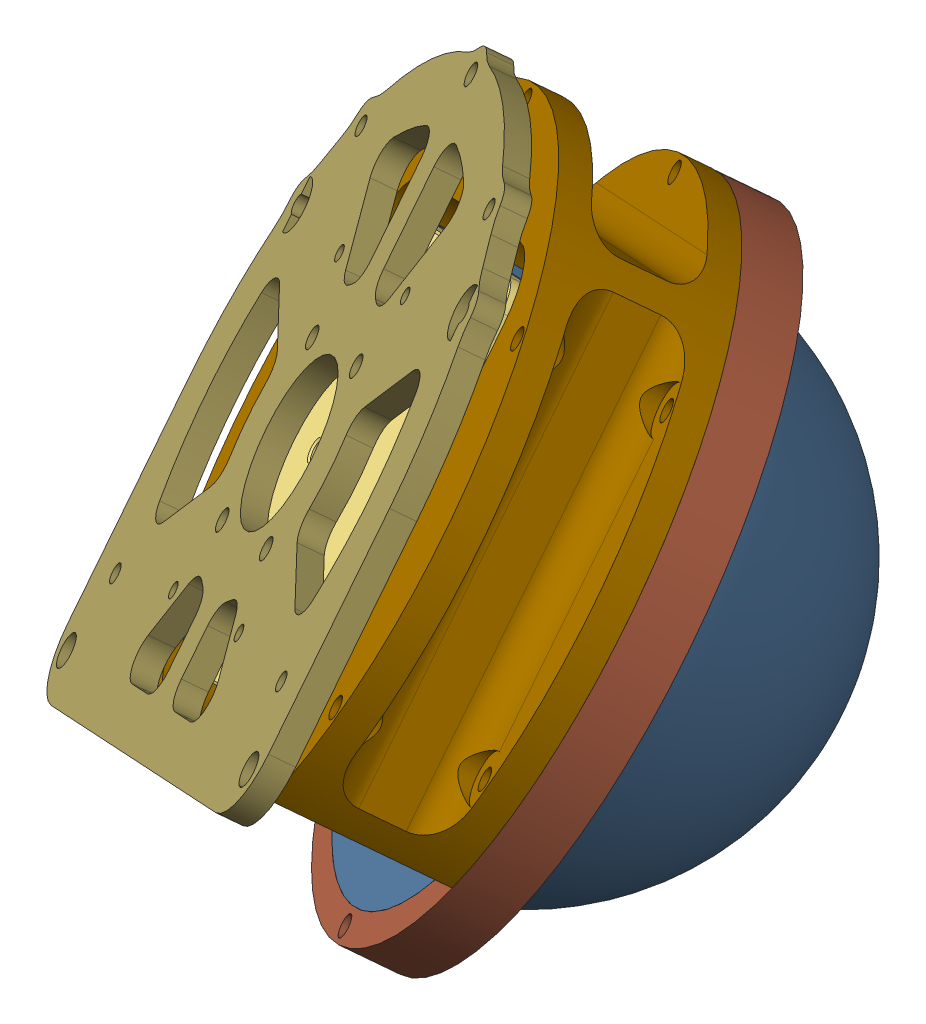
SolidWorks assembly MID装配, configuration 默认. Lengths in mm.
Overall size (2051.22 2631.75 2584.86).
22 component instances, 17 part files, 24 mates.
Components (placement in the parent):
- mid-360-fov-asm (1)-1: mid-360-fov-asm (1) [默认] at (17.2226 -18.313 -129.1674) x (0.033606 -0.751787 0.658549) z (0.781275 0.430686 0.451795) size (1865.26 855.73 1862.57)
  - MID-360_4_ASM_2_ASM-1: MID-360_4_ASM_2_ASM [默认] at origin size (72.74 69.7 66.83)
    - MID-360_4_ASM_2_ASM-1: MID-360_4_ASM_2_ASM [默认] at origin size (71.74 36.3 66.83)
    - MID-360_4_1_1-1: MID-360_4_1_1 [默认] at origin size (52.18 60.17 55.44)
    - MID-360_4_2_1-1: MID-360_4_2_1 [默认] at origin size (64.79 8.1 64.79)
    - MID-360_4_3_2-1: MID-360_4_3_2 [默认] at origin size (13.8 16 22)
    - MID-360_4_4_1-1: MID-360_4_4_1 [默认] at origin size (0.41 0.13 0.13)
    - MID-360_4_5_1-1: MID-360_4_5_1 [默认] at origin size (0.41 0.13 0.13)
    - MID-360_4_6_1-1: MID-360_4_6_1 [默认] at origin size (0.41 0.13 0.13)
    - MID-360_4_7_1-1: MID-360_4_7_1 [默认] at origin size (0.41 0.13 0.13)
  - RECEIVE_FOV_MOVE_2-1: RECEIVE_FOV_MOVE_2 [默认] at origin size (1865.26 855.73 1862.57) (hidden)
- MID、IMU安装板-1: MID、IMU安装板 [默认] at (33.8461 -66.424 -112.0507) x (0.781275 0.430686 0.451795) z (-0.623282 0.499325 0.601826) size (110 110 4) (hidden)
- MID_360罩子装配-1: MID_360罩子装配 [默认] at (-81.3117 -131.4051 -186.4402) x (0.689448 -0.012297 0.724231) z (0.369027 0.866328 -0.336594) size (152.25 67.6 152.25)
  - 舱盖固定环-1: 舱盖固定环 [默认] at (108.0224 -30.5011 115.059) x (-0.837169 0 -0.546944) z (0 1 0) size (110 110 9) (hidden)
  - MID_360罩子-1: MID_360罩子 [默认] at (108.0224 -35.5011 115.059) size (99.6 45 99.6) (hidden)
  - 固定法兰-1: 固定法兰 [默认] at (108.0224 -58.1011 115.059) x (0 1 0) z (0 0 1) size (27.6 110 110) (hidden)
- 零件5^MID装配-1: 零件5^MID装配 [默认] at (2.6821 -41.4577 -81.9594) x (-0.781275 -0.430686 -0.451795) z (0.623282 -0.499325 -0.601826) size (110 110 0) (virtual)
- MID保护罩支撑2222-1: MID保护罩支撑2222 [默认] at (2.6821 -41.4577 -81.9594) x (-0.781275 -0.430686 -0.451795) z (0.623282 -0.499325 -0.601826) size (110 95.89 27)
- MID_360罩子-1: MID_360罩子 [默认] at (17.8976 -18.8537 -129.8191) x (0.769682 0.527758 0.35925) z (-0.138236 0.687129 -0.713263) size (99.6 45 99.6)
- 舱盖固定环-1: 舱盖固定环 [默认] at (17.8976 -18.8537 -129.8191) x (-0.781275 -0.430686 -0.451795) z (0.623282 -0.499325 -0.601826) size (110 110 9)
- imu-1: imu [默认] at (-6.4104 0.62 -106.3479) x (0.033606 -0.751787 0.658549) z (0.781275 0.430686 0.451795) size (43.1 8 31.5) (hidden)
- 零件6^MID装配-2: 零件6^MID装配 [默认] at (0.1889 -39.4604 -79.5521) x (0.781275 0.430686 0.451795) z (-0.623282 0.499325 0.601826) size (110 101.5 4) (virtual)
Mates (geometry in assembly coordinates):
- 重合6: coincident anti-aligned: plane of mid-360-fov-asm (1)-1/MID-360_4_ASM_2_ASM-1/MID-360_4_2_1-1 through (1.069 -5.3719 -113.5698) normal (-0.623282 0.499325 0.601826); plane of MID、IMU安装板-1 through (2.6821 -41.4577 -81.9594) normal (0.623282 -0.499325 -0.601826)
- 同心3: concentric anti-aligned: circle of mid-360-fov-asm (1)-1/MID-360_4_ASM_2_ASM-1/MID-360_4_1_1-1; circle of MID、IMU安装板-1
- 同心4: concentric anti-aligned: cylinder of mid-360-fov-asm (1)-1/MID-360_4_ASM_2_ASM-1/MID-360_4_2_1-1 through (-9.0112 -33.7117 -108.9638) axis (-0.623282 0.499325 0.601826) radius 1.25; cylinder of MID、IMU安装板-1 through (-14.6806 -29.1699 -103.4896) axis (0.623282 -0.499325 -0.601826) radius 1.25
- 在位2: in place: plane of ? through (-21.0592 -70.7891 8.6459) normal (-0.207144 -0.432477 -0.877528); plane of ? through (-5.6737 -11.8455 -24.0354) normal (-0.207144 -0.432477 -0.877528); moOrthogonalPlaneRef_w of ? through (-21.0592 -70.7891 8.6459) normal (-0.207144 -0.432477 -0.877528); plane of ? through (-5.6737 -11.8455 -24.0354) normal (0 0.896983 -0.442065); plane of ? through (-21.0592 -70.7891 8.6459) normal (-0.207144 -0.432477 -0.877528); plane of ? through (-5.6737 -11.8455 -24.0354) normal (-0.97831 0.091571 0.185805); plane of MID、IMU安装板-1 through (2.6821 -41.4577 -81.9594) normal (0.623282 -0.499325 -0.601826); unknown of ?
- 重合8: coincident aligned: plane of MID、IMU安装板-1; plane of 零件5^MID装配-1
- 重合9: coincident aligned: moOrthogonalPlaneRef_w of MID、IMU安装板-1; plane of 零件5^MID装配-1 through (2.6821 -41.4577 -81.9594) normal (-0.033606 0.751787 -0.658549)
- 重合10: coincident anti-aligned: moOrthogonalPlaneRef_w of MID、IMU安装板-1; plane of 零件5^MID装配-1 through (2.6821 -41.4577 -81.9594) normal (-0.781275 -0.430686 -0.451795)
- 同心5: concentric aligned: cylinder of MID、IMU安装板-1 through (1.069 -5.3719 -113.5698) axis (-0.623282 0.499325 0.601826) radius 12.5; cylinder of MID_360罩子装配-1/舱盖固定环-1 through (22.2228 -22.3187 -133.9954) axis (-0.623282 0.499325 0.601826) radius 55
- 在位3: in place: plane of ? through (-21.4766 -37.5277 -47.6627) normal (0.623282 -0.499325 -0.601826); plane of ? through (21.2148 -16.9956 -20.4845) normal (0.623282 -0.499325 -0.601826); plane of ? through (-21.4766 -37.5277 -47.6627) normal (0.623282 -0.499325 -0.601826); plane of ? through (21.2148 -16.9956 -20.4845) normal (0.625229 0.780441 0); plane of ? through (-21.4766 -37.5277 -47.6627) normal (0.623282 -0.499325 -0.601826); plane of ? through (21.2148 -16.9956 -20.4845) normal (-0.46969 0.376279 -0.798627); plane of MID、IMU安装板-1 through (2.6821 -41.4577 -81.9594) normal (0.623282 -0.499325 -0.601826); unknown of ?
- 重合16: coincident aligned: plane of MID、IMU安装板-1; plane of MID保护罩支撑2222-1
- 重合17: coincident aligned: moOrthogonalPlaneRef_w of MID、IMU安装板-1 through (2.6821 -41.4577 -81.9594) normal (-0.033606 0.751787 -0.658549); plane of 零件6^MID装配-1 through (2.6821 -41.4577 -81.9594) normal (-0.033606 0.751787 -0.658549)
- 重合18: coincident anti-aligned: moOrthogonalPlaneRef_w of MID、IMU安装板-1 through (2.6821 -41.4577 -81.9594) normal (0.781275 0.430686 0.451795); plane of 零件6^MID装配-1 through (2.6821 -41.4577 -81.9594) normal (-0.781275 -0.430686 -0.451795)
- 同心6: concentric anti-aligned: cylinder of MID_360罩子-1 through (45.9453 -41.3233 -156.9012) axis (0.623282 -0.499325 -0.601826) radius 49.8; cylinder of 舱盖固定环-1 through (23.5071 -23.3476 -135.2355) axis (-0.623282 0.499325 0.601826) radius 55
- 重合19: coincident anti-aligned: plane of MID_360罩子-1 through (-13.4072 -44.9524 -148.8944) normal (0.623282 -0.499325 -0.601826); plane of 舱盖固定环-1 through (57.6017 -1.181 -111.6703) normal (-0.623282 0.499325 0.601826)
- 同心7: concentric aligned: cylinder of MID保护罩支撑2222-1 through (14.7812 -16.3571 -126.8099) axis (-0.623282 0.499325 0.601826) radius 55; cylinder of 舱盖固定环-1 through (23.5071 -23.3476 -135.2355) axis (-0.623282 0.499325 0.601826) radius 55
- 同心8: concentric anti-aligned: cylinder of MID保护罩支撑2222-1 through (-15.6414 -57.3194 -135.3573) axis (-0.623282 0.499325 0.601826) radius 1.5; cylinder of 舱盖固定环-1 through (-15.6414 -57.3194 -135.3573) axis (0.623282 -0.499325 -0.601826) radius 1.55
- 重合20: coincident anti-aligned: plane of MID保护罩支撑2222-1 through (19.5107 -54.9395 -98.2087) normal (0.623282 -0.499325 -0.601826); plane of 舱盖固定环-1 through (17.8976 -18.8537 -129.8191) normal (-0.623282 0.499325 0.601826)
- 重合21: coincident anti-aligned: plane of MID、IMU安装板-1 through (0.1889 -39.4604 -79.5521) normal (-0.623282 0.499325 0.601826); plane of imu-1 through (-1.4241 -3.3746 -111.1625) normal (0.623282 -0.499325 -0.601826)
- 同心9: concentric anti-aligned: cylinder of MID、IMU安装板-1 through (8.4427 -7.9495 -97.1482) axis (0.623282 -0.499325 -0.601826) radius 1.75; cylinder of imu-1 through (8.4427 -7.9495 -97.1482) axis (-0.623282 0.499325 0.601826) radius 1.5
- 同心10: concentric aligned: circle of MID、IMU安装板-1; cylinder of imu-1 through (-10.4173 -18.3463 -108.0545) axis (-0.623282 0.499325 0.601826) radius 1.5
- 在位4: in place: plane of ? through (1.2895 -38.6099 -81.8358) normal (-0.623282 0.499325 0.601826); plane of ? through (43.2143 -34.62 -41.7267) normal (-0.623282 0.499325 0.601826); plane of ? through (1.2895 -38.6099 -81.8358) normal (-0.623282 0.499325 0.601826); plane of ? through (43.2143 -34.62 -41.7267) normal (0.625229 0.780441 0); plane of ? through (1.2895 -38.6099 -81.8358) normal (-0.623282 0.499325 0.601826); plane of ? through (43.2143 -34.62 -41.7267) normal (0.46969 -0.376279 0.798627); plane of MID、IMU安装板-1 through (0.1889 -39.4604 -79.5521) normal (-0.623282 0.499325 0.601826); unknown of 零件6^MID装配-2
- 重合22: coincident aligned: plane of MID、IMU安装板-1; plane of 零件6^MID装配-2
- 重合23: coincident aligned: moOrthogonalPlaneRef_w of MID、IMU安装板-1 through (0.1889 -39.4604 -79.5521) normal (-0.033606 0.751787 -0.658549); plane of 零件6^MID装配-2 through (0.1889 -39.4604 -79.5521) normal (-0.033606 0.751787 -0.658549)
- 重合24: coincident anti-aligned: moOrthogonalPlaneRef_w of MID、IMU安装板-1 through (0.1889 -39.4604 -79.5521) normal (-0.781275 -0.430686 -0.451795); plane of 零件6^MID装配-2 through (0.1889 -39.4604 -79.5521) normal (0.781275 0.430686 0.451795)
